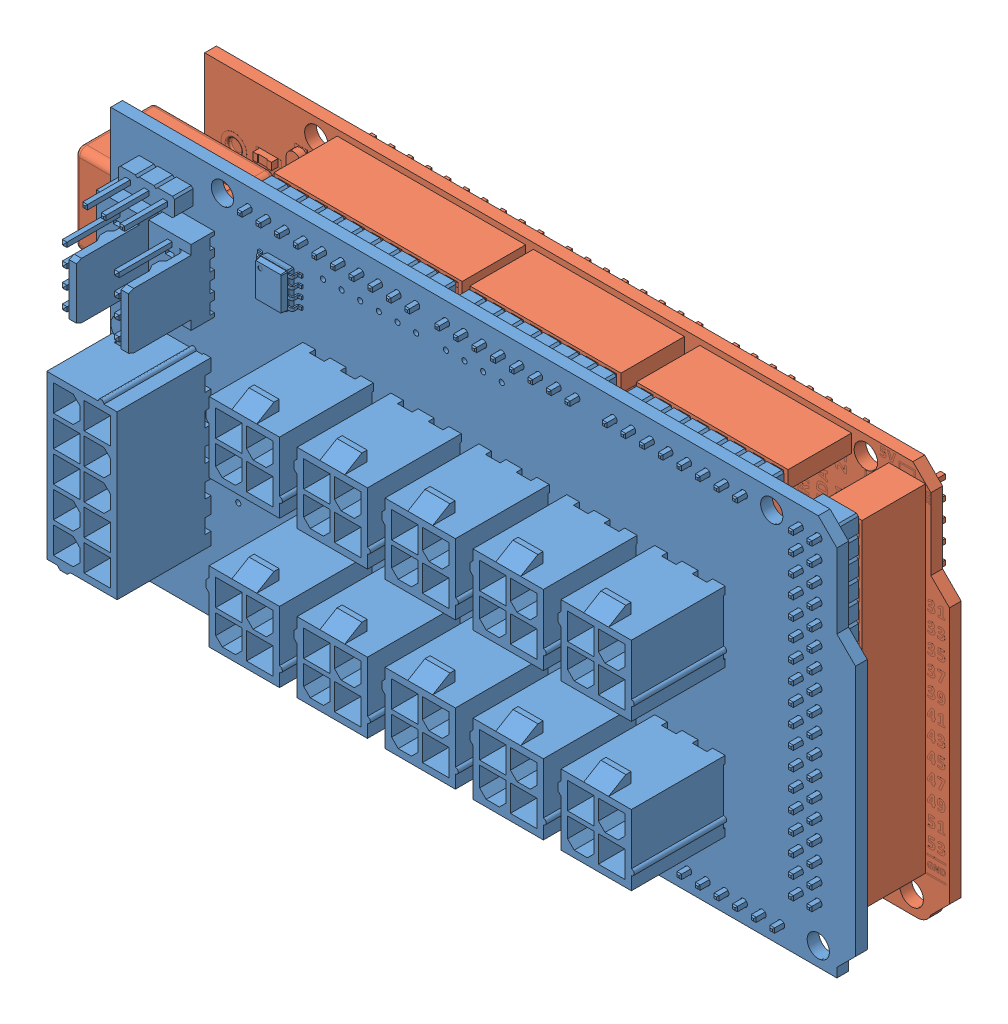
SolidWorks assembly Assem39, configuration Default. Lengths in mm.
Overall size (108.38 53.6 29.29).
2 component instances, 2 part files, 3 mates.
Components (placement in the parent):
- ABSIS_Backlight_Controller-1: ABSIS_Backlight_Controller [Default] at (-198.1649 -5.0008 60.1107) size (101.6 53.34 23.04)
- Arduino MEGA 2560 R3-1: Arduino MEGA 2560 R3 [Default] at (-147.3901 21.5383 48.8707) x (0 1 0) z (1 0 0) size (53.6 14.61 108.35)
Mates (geometry in assembly coordinates):
- Concentric1: concentric: cylinder of ABSIS_Backlight_Controller-1 through (-107.9949 45.7992 59.3107) axis (0 0 1) radius 1.524; cylinder of Arduino MEGA 2560 R3-1 through (-107.9949 45.7992 19.504) axis (0 0 1) radius 1.6081
- Parallel1: parallel: plane of ABSIS_Backlight_Controller-1 through (-198.1649 48.3392 60.1107) normal (0 1 0); plane of Arduino MEGA 2560 R3-1 through (-198.1901 48.3383 19.504) normal (0 1 0)
- Coincident1: coincident anti-aligned: plane of ABSIS_Backlight_Controller-1 through (-167.9389 45.7992 57.5207) normal (0 0 -1); plane of Arduino MEGA 2560 R3-1 through (-147.3901 21.5383 29.754) normal (0 0 1)
